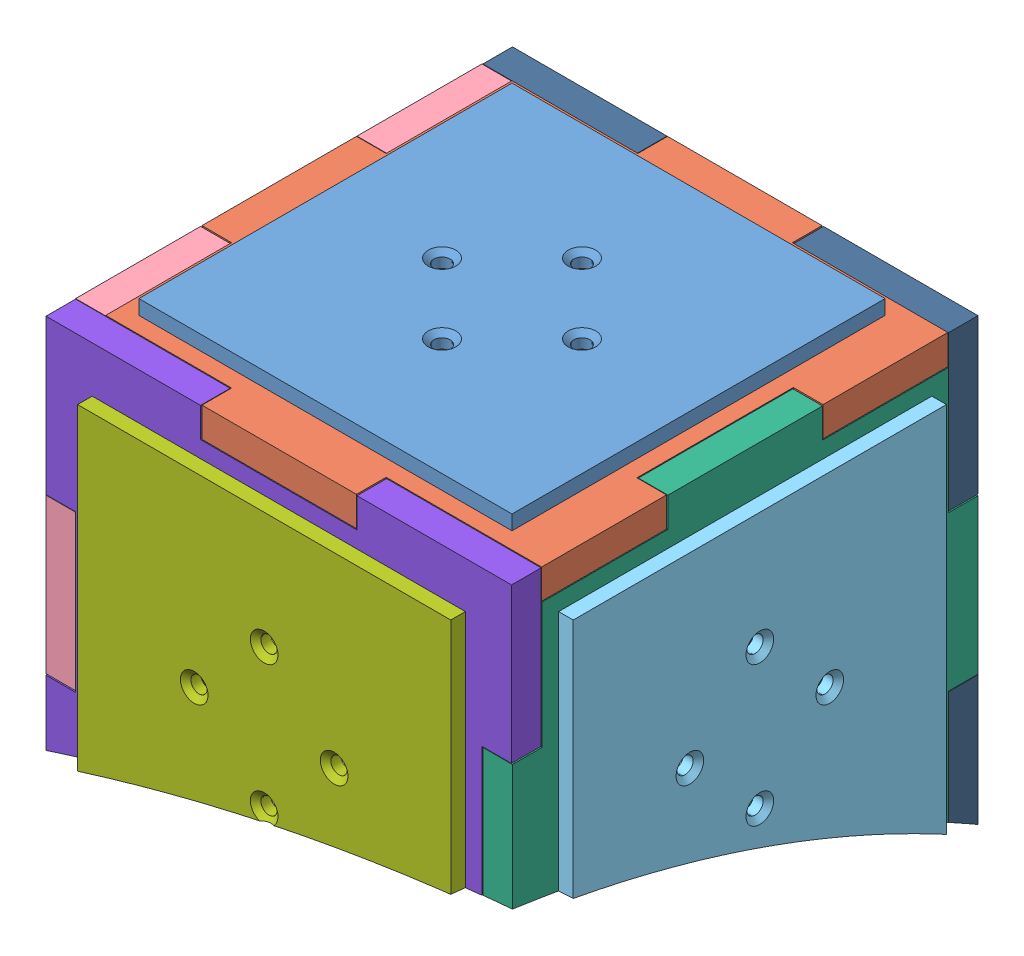
SolidWorks assembly cube_10, configuration cube10. Lengths in mm.
Overall size (53.98 55.56 54.09).
12 component instances, 12 part files, 6 mates.
Components (placement in the parent):
- panel_R^cube_10-13: panel_R^cube_10 [cube01] x (-1 0 0) z (0 0 1) size (40.64 1.59 40.64) (virtual)
- acrylic_R^cube_10-1: acrylic_R^cube_10 [A] at origin size (50.7 3.23 50.7) (virtual)
- panel_O^cube_10-8: panel_O^cube_10 [cube01] x (0 -1 0) z (0 0 1) size (40.92 1.59 40.64) (virtual)
- acrylic_O^cube_10-23: acrylic_O^cube_10 [A] x (0 1 0) z (0 0 1) size (47.97 3.23 50.7) (virtual)
- panel_Y^cube_10-9: panel_Y^cube_10 [cube01] at origin size (40.64 1.59 40.64) (suppressed, hidden, virtual)
- acrylic_Y^cube_10-24: acrylic_Y^cube_10 [A] x (-1 0 0) z (0 0 1) size (50.7 3.23 50.7) (suppressed, hidden, virtual)
- panel_G^cube_10-10: panel_G^cube_10 [cube01] x (0 1 0) z (0 0 1) size (40.54 1.59 40.64) (virtual)
- acrylic_G^cube_10-25: acrylic_G^cube_10 [A] x (0 -1 0) z (0 0 1) size (46.16 3.23 50.7) (virtual)
- panel_C^cube_10-11: panel_C^cube_10 [cube01] x (-1 0 0) z (0 -1 0) size (40.64 1.7 37.32) (virtual)
- acrylic_C^cube_10-26: acrylic_C^cube_10 [B] x (1 0 0) z (0 -1 0) size (50.7 3.23 40.96) (virtual)
- panel_B^cube_10-13: panel_B^cube_10 [cube01] x (-1 0 0) z (0 1 0) size (40.64 1.59 47.37) (virtual)
- acrylic_B^cube_10-27: acrylic_B^cube_10 [B] x (1 0 0) z (0 1 0) size (50.7 3.23 53.92) (virtual)
Mates (geometry in assembly coordinates):
- Coincident1: coincident aligned: plane of panel_R^cube_10-13 through (0 0 0) normal (0 0 1); plane of assembly through (0 0 0) normal (0 0 1)
- Coincident2: coincident anti-aligned: plane of panel_R^cube_10-13; plane of assembly through (0 0 0) normal (1 0 0)
- Coincident3: coincident anti-aligned: plane of panel_R^cube_10-13; plane of assembly through (0 0 0) normal (0 1 0)
- Coincident4: coincident aligned: plane of acrylic_R^cube_10-1 through (0 0 0) normal (0 0 1); plane of assembly through (0 0 0) normal (0 0 1)
- Coincident5: coincident aligned: plane of acrylic_R^cube_10-1 through (0 0 0) normal (1 0 0); plane of assembly through (0 0 0) normal (1 0 0)
- Coincident6: coincident aligned: plane of ? through (0 0 0) normal (0 1 0); plane of assembly through (0 0 0) normal (0 1 0)
